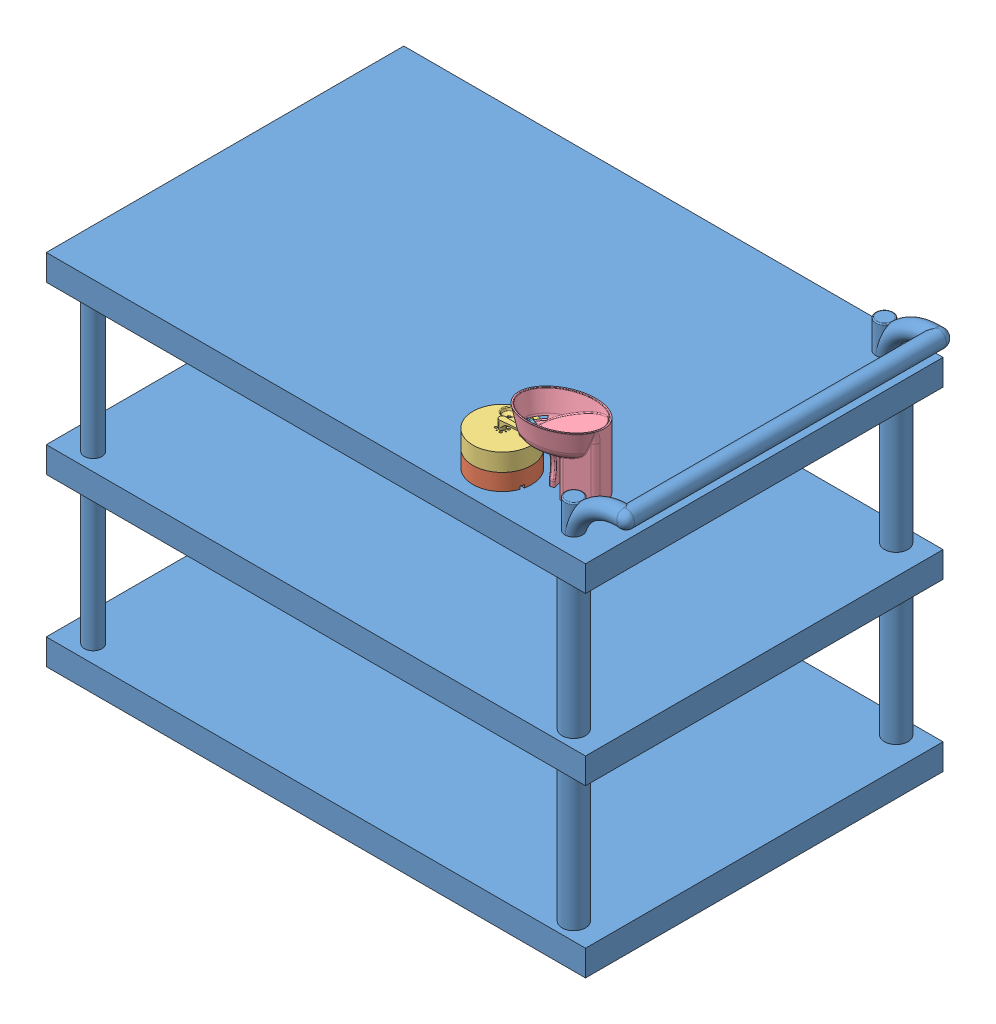
SolidWorks assembly 2-오목알 case랑 디스펜서 각도 체크용 어셈, configuration Default. Lengths in mm.
Overall size (964.58 726.73 610).
6 component instances, 5 part files, 9 mates.
Components (placement in the parent):
- Cart-1: Cart [Default] at origin size (964.58 691.89 610)
- Motor fixed flat-1: Motor fixed flat [Default] at (247 606.3 234) size (100 28.3 100)
- 입X_Rotating plate-1: 입X_Rotating plate [Default] at (247 640.3 234) x (0.850029 0 -0.526735) z (0.526735 0 0.850029) size (100 44.77 100)
- 입X_stone case-1: 입X_stone case [Default] at (322.3933 722 208.4227) x (0.96189 0 -0.273438) z (0.273438 0 0.96189) size (138.78 114.73 102)
- 알-1: 알 [Default] at (279.2035 683.6152 224.5802) x (-0.212887 0.976537 0.032491) z (-0.953609 -0.214903 0.210826) size (19 7.5 19)
- 알-2: 알 [Default] at (277.2441 680.9028 216.7465) x (-0.554696 0.827027 0.091314) z (0.813891 0.562116 -0.146997) size (19 7.5 19)
Mates (geometry in assembly coordinates):
- 일치3: coincident anti-aligned: plane of Motor fixed flat-1 through (247 640.3 234) normal (0 1 0); plane of Rotating plate-1 through (247 640.3 234) normal (0 -1 0)
- 일치5: coincident anti-aligned: plane of Cart-1 through (0 612 0) normal (0 1 0); plane of Motor fixed flat-1 through (247 612 234) normal (0 -1 0)
- 동심2: concentric anti-aligned: cylinder of Motor fixed flat-1 through (247 605 234) axis (0 1 0) radius 50; cylinder of Rotating plate-1 through (247 670.3 234) axis (0 -1 0) radius 50
- 거리4: distance = 213 mm: cylinder of Rotating plate-1 through (247 682.07 234) axis (0 -1 0) radius 5; plane of Cart-1 through (460 612 305) normal (1 0 0)
- 거리5: distance = 71 mm: cylinder of Rotating plate-1 through (247 682.07 234) axis (0 -1 0) radius 5; plane of Cart-1 through (-460 612 305) normal (0 0 1)
- 거리6: distance = 74 mm: cylinder of 입X_stone case-1 through (360 617 231) axis (0 -1 0) radius 2.5; plane of Cart-1 through (-460 612 305) normal (0 0 1)
- 거리7: distance = 100 mm: cylinder of 입X_stone case-1 through (360 617 231) axis (0 -1 0) radius 2.5; plane of Cart-1 through (460 612 305) normal (1 0 0)
- 일치4: coincident anti-aligned: plane of Cart-1 through (0 612 0) normal (0 1 0); plane of 입X_stone case-1 through (322.3933 612 208.4227) normal (0 -1 0)
- 거리8: distance = 117.5 mm: plane of Cart-1 through (460 612 305) normal (1 0 0); cylinder of 입X_stone case-1 through (342.5 617 169.4391) axis (0 -1 0) radius 2.5
